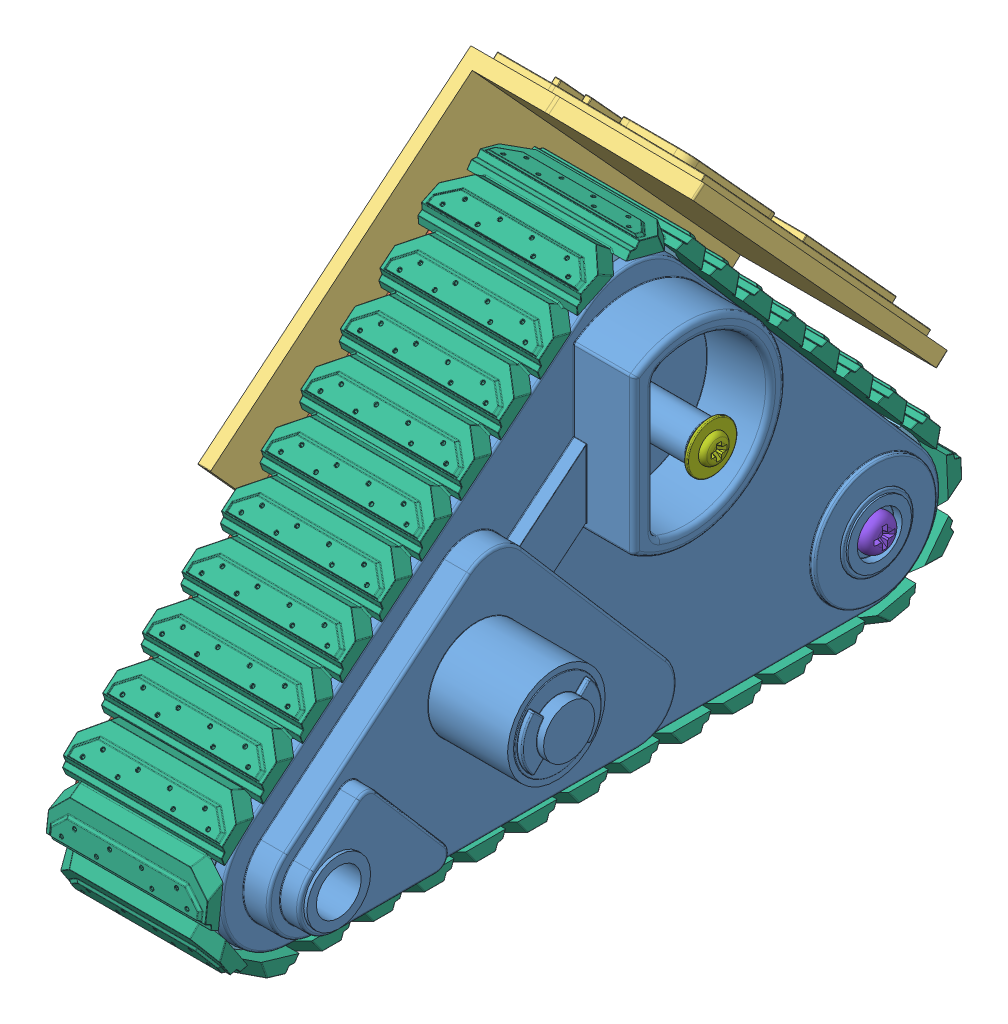
SolidWorks assembly TDRV (Right), configuration Default. Lengths in mm.
Overall size (51.05 82.74 123.21).
17 component instances, 8 part files, 33 mates.
Components (placement in the parent):
- Track Drive Side (Right, Inner)-1: Track Drive Side (Right, Inner) [Default] at (11.975 -11 -45.5) size (22.2 65.97 113)
- Track Drive Side (Right, Outer)-1: Track Drive Side (Right, Outer) [Default] at (-11.975 -11 -45.5) size (26.75 65.97 113)
- TDRV Beauty Cover (Right)-1: TDRV Beauty Cover (Right) [Default] at (-20.575 -4.6199 -48.4187) x (1 0 0) z (0 -0.001763 0.999998) size (32.9 69.17 84.78)
- Roller-1: Roller [Default] x (-1 0 0) z (0 0.637242 -0.770664) size (18.92 25.7 25.7)
  - Roller (Female)-1: Roller (Female) [Default] at (5.16 0 0) size (10.22 25.7 25.7)
  - Roller (Male)-1: Roller (Male) [Default] at (-5.16 0 0) size (13 25.7 25.7)
- Roller-3: Roller [Default] at (0 0 -91) x (-1 0 0) z (0 -1 0) size (18.92 25.7 25.7)
  - Roller (Female)-1: Roller (Female) [Default] at (5.16 0 0) size (10.22 25.7 25.7)
  - Roller (Male)-1: Roller (Male) [Default] at (-5.16 0 0) size (13 25.7 25.7)
- Roller-2: Roller [Default] at (0 43.9697 -53.1758) x (-1 0 0) z (0 -0.637242 0.770664) size (18.92 25.7 25.7)
  - Roller (Female)-1: Roller (Female) [Default] at (5.16 0 0) size (10.22 25.7 25.7)
  - Roller (Male)-1: Roller (Male) [Default] at (-5.16 0 0) size (13 25.7 25.7)
- Treads-1: Treads [Default] at (0 -11 -45.5) size (25 72.41 119.4)
- Washer Head Thread-Forming Screw 2.6mm x 6mm-1: Washer Head Thread-Forming Screw 2.6mm x 6mm [Default] at (18.575 36.4697 -53.1758) x (0 -1 0) z (0 0 1) size (7.8 7.44 7.8)
- Cheese Head Thread-Forming Screw 2.8mm x 8mm-1: Cheese Head Thread-Forming Screw 2.8mm x 8mm [Default] at (4.275 0 0) x (0 -1 0) z (0 0 1) size (5.45 9.97 5.45)
- Cheese Head Thread-Forming Screw 2.8mm x 8mm-5: Cheese Head Thread-Forming Screw 2.8mm x 8mm [Default] at (4.275 0 -91) x (0 -1 0) z (0 0 1) size (5.45 9.97 5.45)
- Cheese Head Thread-Forming Screw 2.8mm x 8mm-6: Cheese Head Thread-Forming Screw 2.8mm x 8mm [Default] at (4.275 43.9697 -53.1758) x (0 -1 0) z (0 0 1) size (5.45 9.97 5.45)
Mates (geometry in assembly coordinates):
- Concentric1: concentric: cylinder of Track Drive Side (Right, Inner)-1 through (11.975 0 0) axis (-1 0 0) radius 1.7; cylinder of Track Drive Side (Right, Outer)-1 through (39.5931 0 0) axis (-1 0 0) radius 3.1
- Coincident1: coincident: plane of Track Drive Side (Right, Inner)-1 through (10.275 -11 -45.5) normal (-1 0 0); plane of Track Drive Side (Right, Outer)-1 through (10.275 -11 -45.5) normal (1 0 0)
- Concentric2: concentric: cylinder of Track Drive Side (Right, Inner)-1 through (11.975 0 -91) axis (-1 0 0) radius 1.7; cylinder of Track Drive Side (Right, Outer)-1 through (39.5931 0 -91) axis (-1 0 0) radius 3.1
- Concentric3: concentric: cylinder of Track Drive Side (Right, Inner)-1 through (44.8171 0 0) axis (-1 0 0) radius 3.525; point of assembly
- Parallel1: parallel: plane of Track Drive Side (Right, Inner)-1 through (11.975 -11 -45.5) normal (0 1 0); plane of assembly through (0 0 0) normal (0 1 0)
- Symmetric1: symmetric aligned: plane of Track Drive Side (Right, Inner)-1 through (11.975 -11 -45.5) normal (1 0 0); plane of Track Drive Side (Right, Outer)-1 through (-11.975 -11 -45.5) normal (-1 0 0); plane of assembly through (0 0 0) normal (1 0 0)
- Concentric4: concentric aligned: cylinder of Track Drive Side (Right, Inner)-1 through (11.975 0 0) axis (-1 0 0) radius 1.7; cylinder of Roller-1/Roller (Male)-1 through (9.46 0 0) axis (-1 0 0) radius 3.5
- Concentric5: concentric aligned: cylinder of Track Drive Side (Right, Inner)-1 through (11.975 0 -91) axis (-1 0 0) radius 1.7; cylinder of Roller-3/Roller (Male)-1 through (9.46 0 -91) axis (-1 0 0) radius 3.5
- Concentric6: concentric aligned: cylinder of Track Drive Side (Right, Inner)-1 through (11.975 43.9697 -53.1758) axis (-1 0 0) radius 1.7; cylinder of Roller-2/Roller (Male)-1 through (9.46 43.9697 -53.1758) axis (-1 0 0) radius 3.5
- Coincident3: coincident anti-aligned: plane of Roller-1; plane of assembly through (0 0 0) normal (1 0 0)
- Coincident5: coincident anti-aligned: plane of Roller-3; plane of assembly through (0 0 0) normal (1 0 0)
- Coincident4: coincident anti-aligned: plane of Roller-2; plane of assembly through (0 0 0) normal (1 0 0)
- Coincident6: coincident anti-aligned: plane of Track Drive Side (Right, Outer)-1 through (-16.475 12.3697 -42.5013) normal (-1 0 0); plane of TDRV Beauty Cover (Right)-1 through (-16.475 -4.6199 -48.4187) normal (1 0 0)
- Concentric7: concentric aligned: cylinder of Track Drive Side (Right, Outer)-1 through (10.275 12.3697 -42.5013) axis (-1 0 0) radius 1.6; cylinder of TDRV Beauty Cover (Right)-1 through (1.2676 12.3697 -42.5013) axis (-1 0 0) radius 1.5
- Concentric8: concentric aligned: cylinder of Track Drive Side (Right, Outer)-1 through (10.275 24 -75.088) axis (-1 0 0) radius 1.6; cylinder of TDRV Beauty Cover (Right)-1 through (1.2676 24 -75.088) axis (-1 0 0) radius 1.5
- Concentric9: concentric aligned: cylinder of Track Drive Side (Right, Inner)-1 through (23.675 36.4697 -53.1758) axis (1 0 0) radius 0.8; cylinder of Washer Head Thread-Forming Screw 2.6mm x 6mm-1 through (25.975 36.4697 -53.1758) axis (1 0 0) radius 1.3
- Distance1: distance = 2.9 mm anti-aligned: plane of Washer Head Thread-Forming Screw 2.6mm x 6mm-1 through (24.375 37.7697 -53.1758) normal (-1 0 0); plane of Track Drive Side (Right, Inner)-1 through (21.475 -11 -45.5) normal (1 0 0)
- Parallel3: parallel anti-aligned: plane of Washer Head Thread-Forming Screw 2.6mm x 6mm-1; plane of assembly through (0 0 0) normal (0 1 0)
- Concentric11: concentric aligned: cylinder of Track Drive Side (Right, Outer)-1 through (10.275 0 0) axis (1 0 0) radius 0.9; cylinder of Cheese Head Thread-Forming Screw 2.8mm x 8mm-1 through (14.175 0 0) axis (1 0 0) radius 1.4
- Coincident8: coincident anti-aligned: plane of Track Drive Side (Right, Inner)-1 through (11.975 -11 -45.5) normal (1 0 0); plane of Cheese Head Thread-Forming Screw 2.8mm x 8mm-1 through (11.975 1.4 0) normal (-1 0 0)
- Parallel6: parallel anti-aligned: plane of Cheese Head Thread-Forming Screw 2.8mm x 8mm-1; plane of assembly through (0 0 0) normal (0 1 0)
- Parallel7: parallel anti-aligned: plane of Cheese Head Thread-Forming Screw 2.8mm x 8mm-5; plane of assembly through (0 0 0) normal (0 1 0)
- Concentric12: concentric aligned: cylinder of Track Drive Side (Right, Outer)-1 through (10.275 0 -91) axis (1 0 0) radius 0.9; cylinder of Cheese Head Thread-Forming Screw 2.8mm x 8mm-5 through (14.175 0 -91) axis (1 0 0) radius 1.4
- Coincident9: coincident anti-aligned: plane of Track Drive Side (Right, Inner)-1 through (11.975 -11 -45.5) normal (1 0 0); plane of Cheese Head Thread-Forming Screw 2.8mm x 8mm-5 through (11.975 1.4 -91) normal (-1 0 0)
- Concentric13: concentric aligned: cylinder of Track Drive Side (Right, Outer)-1 through (10.275 43.9697 -53.1758) axis (1 0 0) radius 0.9; cylinder of Cheese Head Thread-Forming Screw 2.8mm x 8mm-6 through (14.175 43.9697 -53.1758) axis (1 0 0) radius 1.4
- Parallel8: parallel anti-aligned: plane of Cheese Head Thread-Forming Screw 2.8mm x 8mm-6; plane of assembly through (0 0 0) normal (0 1 0)
- Coincident10: coincident anti-aligned: plane of Track Drive Side (Right, Inner)-1 through (11.975 -11 -45.5) normal (1 0 0); plane of Cheese Head Thread-Forming Screw 2.8mm x 8mm-6 through (11.975 45.3697 -53.1758) normal (-1 0 0)
- Coincident11: coincident aligned: plane of Treads-1 through (0 -11 -45.5) normal (1 0 0); plane of assembly through (0 0 0) normal (1 0 0)
- Concentric14: concentric anti-aligned: cylinder of Track Drive Side (Right, Inner)-1 through (44.8171 0 0) axis (-1 0 0) radius 3.525; circle of Treads-1
- Concentric15: concentric anti-aligned: cylinder of Track Drive Side (Right, Inner)-1 through (32.5371 0 -91) axis (-1 0 0) radius 3.525; circle of Treads-1
- Parallel9: parallel aligned: plane of Track Drive Side (Right, Outer)-1 through (-54.164 20.9608 -19.0724) normal (0 0.770664 0.637242); plane of Roller-1
- Parallel10: parallel anti-aligned: plane of Roller-3 through (0 0 -91) normal (0 -1 0); plane of assembly through (0 0 0) normal (0 1 0)
- Parallel11: parallel anti-aligned: plane of Track Drive Side (Right, Outer)-1 through (-54.164 20.9608 -19.0724) normal (0 0.770664 0.637242); plane of Roller-2
